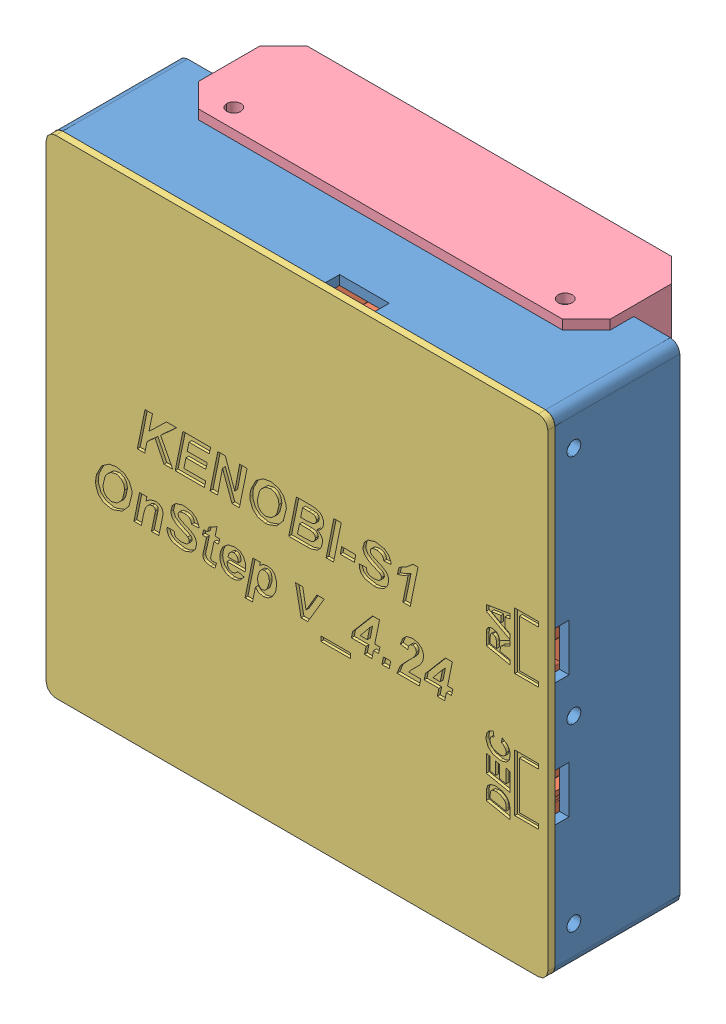
SolidWorks assembly OnStep, configuration По умолчанию. Lengths in mm.
Overall size (106 107 40.9).
4 component instances, 4 part files, 9 mates.
Components (placement in the parent):
- Korp_02-1: Korp_02 [По умолчанию] at origin size (106 103 26.4)
- OneStep_board-1: OneStep_board [По умолчанию] at (50 -48.5 5) x (-1 0 0) z (0 0 -1) size (99.99 97.95 22.03)
- TOP-1: TOP [По умолчанию] at (0 0 26.5) x (-1 0 0) z (0 0 -1) size (106 103 9.5)
- Kr-1: Kr [По умолчанию] at (-0.246 -8.5 -14.4) x (-1 0 0) z (0 1 0) size (87 23 62)
Mates (geometry in assembly coordinates):
- Концентричный2: concentric anti-aligned: cylinder of Korp_01-1 through (-45 39.5 5) axis (0 0 -1) radius 1.35; cylinder of OneStep_board-1 through (-45 39.5 6.6) axis (0 0 1) radius 1.75
- Концентричный3: concentric anti-aligned: cylinder of Korp_01-1 through (45 -43.5 5) axis (0 0 -1) radius 1.35; cylinder of OneStep_board-1 through (45 -43.5 6.6) axis (0 0 1) radius 1.75
- Концентричный4: concentric aligned: cylinder of Korp_01-1 through (-53 43.5 21) axis (1 0 0) radius 1.5; cylinder of TOP-1 through (-53 43.5 21) axis (1 0 0) radius 1.1
- Совпадение2: coincident anti-aligned: plane of Korp_01-1 through (0 0 25) normal (0 0 1); plane of TOP-1 through (0 0 25) normal (0 0 -1)
- Совпадение3: coincident aligned: plane of Korp_01-1 through (-53 -51.5 25) normal (-1 0 0); plane of TOP-1 through (-53 -51.5 25) normal (-1 0 0)
- Совпадение4: coincident anti-aligned: circle of Korp_01-1; plane of OneStep_board-1 through (49.99 -48.5 5) normal (0 0 -1)
- Совпадение5: coincident anti-aligned: plane of Korp_02-1 through (-53 51.5 25) normal (0 1 0); plane of Kr-1 through (1.8431 51.5 -14.4) normal (0 -1 0)
- Совпадение6: coincident anti-aligned: plane of Korp_02-1 through (0 0 -1.4) normal (0 0 -1); plane of Kr-1 through (45.3431 51.5 -1.4) normal (0 0 1)
- Расстояние1: distance = 8 mm: line of Korp_02-1 through (51 51.5 25) axis (0 0 -1); line of Kr-1 through (43.254 53.5 3.6) axis (0 0 -1)
